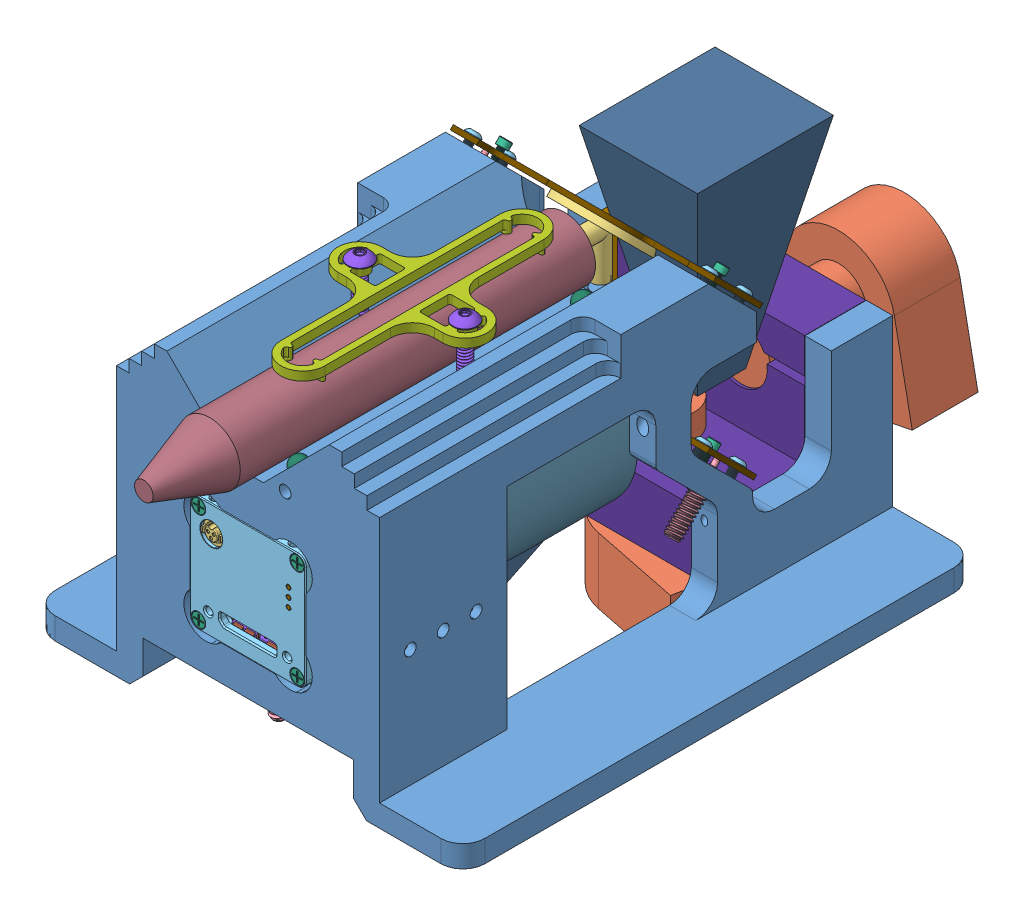
SolidWorks assembly cam_assem, configuration Default. Lengths in mm.
Overall size (98 2576.27 1000).
86 component instances, 46 part files, 77 mates.
Components (placement in the parent):
- cam_holder-1: cam_holder [Default] at origin size (98 71.23 117)
- STP-MQ-(MQ022xG-CM)-ASSM-1: STP-MQ-(MQ022xG-CM)-ASSM [Default] at (0 -13.2 12.4876) x (-1 0 0) z (0 0 -1) size (26.4 26.4 30.19)
  - STP-MQ-(MQ022xG-CM)-ASSM.stp-1: STP-MQ-(MQ022xG-CM)-ASSM.stp [Default] at origin size (26.4 26.4 30.19)
    - SUBASSM-MQ-FRONT.stp-1: SUBASSM-MQ-FRONT.stp [Default] x (0 -1 0) z (0 0 1) size (26.4 26.4 14.6)
      - MECH-MQ-FRONT.stp-1: MECH-MQ-FRONT.stp [Default] at (0 0 7.5) x (1 0 0) z (0 0 -1) size (26.4 26.4 7.5)
      - MECH-MQ-CS-C.stp-1: MECH-MQ-CS-C.stp [Default] at (0 0 0.5) x (1 0 0) z (0 0 -1) size (26.4 26.4 5.5)
      - SROB-M2x14-CUST.stp-1: SROB-M2x14-CUST.stp [Default] at (-11.25 11.25 -7.1) size (3 3 14.55)
      - SROB-M2x14-CUST.stp-2: SROB-M2x14-CUST.stp [Default] at (11.25 -11.25 -7.1) size (3 3 14.55)
      - SROB-M2x14-CUST.stp-3: SROB-M2x14-CUST.stp [Default] at (11.25 11.25 -7.1) size (3 3 14.55)
      - SROB-M2x14-CUST.stp-4: SROB-M2x14-CUST.stp [Default] at (-11.25 -11.25 -7.1) size (3 3 14.55)
    - SUBASSM-MQ-REAR.stp-1: SUBASSM-MQ-REAR.stp [Default] at (0 0 -22.584) x (-1 0 0) z (0 0 1) size (26.4 26.4 10.6)
      - MECH-MQ-REAR.stp-1: MECH-MQ-REAR.stp [Default] at (0 0 6.5) x (-1 0 0) z (0 0 -1) size (26.4 26.4 6.5)
      - SROB-M2x10-CUST .stp-1: SROB-M2x10-CUST .stp [Default] at (-11.25 11.25 10.6) x (1 0 0) z (0 0 -1) size (3 3 10.55)
      - SROB-M2x10-CUST .stp-2: SROB-M2x10-CUST .stp [Default] at (11.25 11.25 10.6) x (1 0 0) z (0 0 -1) size (3 3 10.55)
      - SROB-M2x10-CUST .stp-3: SROB-M2x10-CUST .stp [Default] at (11.25 -11.25 10.6) x (1 0 0) z (0 0 -1) size (3 3 10.55)
      - SROB-M2x10-CUST .stp-4: SROB-M2x10-CUST .stp [Default] at (-11.25 -11.25 10.6) x (1 0 0) z (0 0 -1) size (3 3 10.55)
      - MECH-MQ-THERMAL-PAD.stp-1: MECH-MQ-THERMAL-PAD.stp [Default] at (-10.5 5.45 4.8) x (0.961741 -0.273959 0) z (0 0 -1) size (20.28 8 0.5)
      - MECH-EMI-GSKT-1.3X2.3X11.stp-1: MECH-EMI-GSKT-1.3X2.3X11.stp [Default] at (0 9.9495 3.45) size (11 1.2 3)
      - MECH-EMI-GSKT-1.3X2.3X11.stp-2: MECH-EMI-GSKT-1.3X2.3X11.stp [Default] at (0 7.0505 3.45) size (11 1.2 3)
      - MECH-LIGHTPIPE-1.63X4.14.stp-1: MECH-LIGHTPIPE-1.63X4.14.stp [Default] at (9.3 -3.5 4.1492) x (-1 0 0) z (0 -1 0) size (1.63 4.14 1.63)
      - MECH-LIGHTPIPE-1.63X4.14.stp-2: MECH-LIGHTPIPE-1.63X4.14.stp [Default] at (9.3 -1.5 4.1492) x (-1 0 0) z (0 -1 0) size (1.63 4.14 1.63)
      - MECH-LIGHTPIPE-1.63X4.14.stp-3: MECH-LIGHTPIPE-1.63X4.14.stp [Default] at (9.3 -5.5 4.1492) x (-1 0 0) z (0 -1 0) size (1.63 4.14 1.63)
    - SUBASSM-MQ-MID-022-CM.stp-1: SUBASSM-MQ-MID-022-CM.stp [Default] at (0 0 -4.5) x (-1 0 0) z (0 0 -1) size (26.4 26.4 11.68)
      - MECH-MQ-MID-022-CM-REV2.stp-1: MECH-MQ-MID-022-CM-REV2.stp [Default] at origin size (26.4 26.4 11.59)
      - MECH-O-RING-22X1-VI370.stp-1: MECH-O-RING-22X1-VI370.stp [Default] at (0 0 1.3) x (1 0 0) z (0 1 0) size (24 1 24)
      - FLT-BK7-AR2X-D25.stp-1: FLT-BK7-AR2X-D25.stp [Default] at (0 0 -0.1) size (25 25 1.1)
      - MECH-MX022xG-CM-GSKT.stp-1: MECH-MX022xG-CM-GSKT.stp [Default] at (0 0 3.364) x (0 -1 0) z (0 0 1) size (12.2 17.4 1.27)
    - MQ022xG-CM-PCA-LW_MODEL.stp-1: MQ022xG-CM-PCA-LW_MODEL.stp [Default] at (0 0 -16.486) x (-1 0 0) z (0 0 -1) size (25.43 25.43 13.85)
      - CMV2000.stp-1: CMV2000.stp [Default] at (-0.0259 -0.5261 -1.002) x (-1 0 0) z (0 0 -1) size (18.65 13.5 6.65)
        - ANDON-96UPGA-Socket.stp-1: ANDON-96UPGA-Socket.stp [Default] at origin size (15.9 10.8 3.23)
        - CMV2000_Package.stp-1: CMV2000_Package.stp [Default] at (0 0 3.29) x (-1 0 0) z (0 0 1) size (18.65 13.5 5.45)
        - CMV2000_Glass.stp-1: CMV2000_Glass.stp [Default] at (0 0 6.1) size (18.06 12.95 0.55)
      - MQ022xG-CM-PCA-LW_MODEL-0.stp-1: MQ022xG-CM-PCA-LW_MODEL-0.stp [Default] at origin size (0.25 1.57 4.1)
      - MQ022xG-CM-PCA-LW_MODEL-1.stp-1: MQ022xG-CM-PCA-LW_MODEL-1.stp [Default] at origin size (12.85 2.05 3.8)
      - MQ022xG-CM-PCA-LW_MODEL-2.stp-1: MQ022xG-CM-PCA-LW_MODEL-2.stp [Default] at origin size (25.43 25.43 1)
      - MQ022xG-CM-PCA-LW_MODEL-3.stp-1: MQ022xG-CM-PCA-LW_MODEL-3.stp [Default] at origin size (0.25 1.57 4.1)
      - MQ022xG-CM-PCA-LW_MODEL-4.stp-1: MQ022xG-CM-PCA-LW_MODEL-4.stp [Default] at origin size (5 5 8.1)
      - MQ022xG-CM-PCA-LW_MODEL-5.stp-1: MQ022xG-CM-PCA-LW_MODEL-5.stp [Default] at origin size (0.25 1.57 4.1)
      - MQ022xG-CM-PCA-LW_MODEL-6.stp-1: MQ022xG-CM-PCA-LW_MODEL-6.stp [Default] at origin size (0.25 1.57 4.1)
      - MQ022xG-CM-PCA-LW_MODEL-7.stp-1: MQ022xG-CM-PCA-LW_MODEL-7.stp [Default] at origin size (0.25 1.57 4.1)
      - MQ022xG-CM-PCA-LW_MODEL-8.stp-1: MQ022xG-CM-PCA-LW_MODEL-8.stp [Default] at origin size (0.25 1.57 4.1)
      - MQ022xG-CM-PCA-LW_MODEL-9.stp-1: MQ022xG-CM-PCA-LW_MODEL-9.stp [Default] at origin size (0.25 1.57 4.1)
      - MQ022xG-CM-PCA-LW_MODEL-10.stp-1: MQ022xG-CM-PCA-LW_MODEL-10.stp [Default] at origin size (0.25 1.57 4.1)
      - MQ022xG-CM-PCA-LW_MODEL-11.stp-1: MQ022xG-CM-PCA-LW_MODEL-11.stp [Default] at origin size (0.25 1.57 4.1)
      - MQ022xG-CM-PCA-LW_MODEL-12.stp-1: MQ022xG-CM-PCA-LW_MODEL-12.stp [Default] at origin size (13.8 3 5.6)
      - MQ022xG-CM-PCA-LW_MODEL-13.stp-1: MQ022xG-CM-PCA-LW_MODEL-13.stp [Default] at origin size (0.25 1.57 4.1)
- laser-1: laser [Default] at (0 18.5208 -37.2385) x (0 -1 0) z (0 0 1) size (14 14 96)
- lens-1: lens [Default] at (0 -13.2 -37.0124) x (0 1 0) z (0 0 1) size (33.5 33.5 46.47)
- 1598K25_Hardened Bearing-Quality 440C Stainless Steel Ball-1: 1598K25_Hardened Bearing-Quality 440C Stainless Steel Ball [1598K25] at (-6.6608 12.5671 30) x (0.595435 0.636273 0.490525) z (-0.571952 -0.093063 0.814991) size (4 4 4)
- 92695A729_Alloy Steel Cone-Point Set Screws-1: 92695A729_Alloy Steel Cone-Point Set Screws [92695A729] at (-8.4853 10.8376 24.4029) x (0.913011 -0.407935 0) z (0 0 1) size (4.05 3.54 3.43)
- 1598K25_Hardened Bearing-Quality 440C Stainless Steel Ball-2: 1598K25_Hardened Bearing-Quality 440C Stainless Steel Ball [1598K25] at (-6.364 12.1569 -35) x (0.756378 0.1991 0.623098) z (-0.446406 -0.539153 0.714168) size (4 4 4)
- 1598K25_Hardened Bearing-Quality 440C Stainless Steel Ball-4: 1598K25_Hardened Bearing-Quality 440C Stainless Steel Ball [1598K25] at (6.364 12.1569 -35) x (0.295652 0.723786 0.623477) z (-0.259043 -0.567459 0.781593) size (4 4 4)
- galvo_block-1: galvo_block [Default] at (-18.725 -27.865 -82) x (0 -1 0) z (1 0 0) size (39.65 34.73 42.65)
- D_holder-1: D_holder [Default] at (0 -12.8464 -45.6926) x (1 0 0) z (0 -0.707107 0.707107) size (60 27.4 1)
- D-1: D [Default] at (0 -13.2 -45.339) x (1 0 0) z (0 -0.707107 0.707107) size (20 121.63 78.36)
- glavo-1: glavo [Default] at (0 -59.1765 -60.255) x (0.199368 0 -0.979925) z (0.979925 0 0.199368) size (26 51 34)
- D_holder-2: D_holder [Default] at (0 20.2886 -47.1068) x (1 0 0) z (0 -0.707107 0.707107) size (60 27.4 1)
- mirror-1: mirror [Default] at (0 18.5208 -45.339) x (-1 0 0) z (0 0.707107 -0.707107) size (20 121.63 78.36)
- 3126A21_Slotted Long-Nose Steel Spring Plunger-1: 3126A21_Slotted Long-Nose Steel Spring Plunger [3126A21] at (27 -19.2382 -39.3008) x (0.917455 -0.281315 -0.281315) z (0.397839 0.648739 0.648739) size (3.52 15.42 3.68)
- 92949A319_18-8 Stainless Steel Button Head Hex Drive Screw-1: 92949A319_18-8 Stainless Steel Button Head Hex Drive Screw [92949A319] at (27 -10.9061 -39.8548) x (-0.780279 -0.442247 -0.442247) z (0 0.707107 -0.707107) size (3.28 3.28 7.4)
- 92196A051_18-8 Stainless Steel Socket Head Screw-1: 92196A051_18-8 Stainless Steel Socket Head Screw [92196A051] at (24.75 -13.1743 -45.3647) x (-0.756852 -0.462156 -0.462156) z (0 0.707107 -0.707107) size (2.44 2.44 4.07)
- 92949A319_18-8 Stainless Steel Button Head Hex Drive Screw-2: 92949A319_18-8 Stainless Steel Button Head Hex Drive Screw [92949A319] at (27 -18.6842 -47.633) x (-0.793626 -0.430208 -0.430208) z (0 0.707107 -0.707107) size (3.28 3.28 7.4)
- 92949A319_18-8 Stainless Steel Button Head Hex Drive Screw-3: 92949A319_18-8 Stainless Steel Button Head Hex Drive Screw [92949A319] at (-27 -10.9061 -39.8548) x (-0.831896 -0.392395 -0.392395) z (0 0.707107 -0.707107) size (3.28 3.28 7.4)
- 92949A319_18-8 Stainless Steel Button Head Hex Drive Screw-4: 92949A319_18-8 Stainless Steel Button Head Hex Drive Screw [92949A319] at (-27 -18.6842 -47.633) x (-0.88833 -0.324707 -0.324707) z (0 0.707107 -0.707107) size (3.28 3.28 7.4)
- 92196A051_18-8 Stainless Steel Socket Head Screw-2: 92196A051_18-8 Stainless Steel Socket Head Screw [92196A051] at (-24.75 -13.1164 -45.4227) x (-0.770813 -0.45047 -0.45047) z (0 0.707107 -0.707107) size (2.44 2.44 4.07)
- 3126A21_Slotted Long-Nose Steel Spring Plunger-3: 3126A21_Slotted Long-Nose Steel Spring Plunger [3126A21] at (-27 -19.4685 -39.0705) x (0.908634 -0.295283 -0.295283) z (0.417593 0.642502 0.642502) size (3.52 15.42 3.68)
- 3126A21_Slotted Long-Nose Steel Spring Plunger-5: 3126A21_Slotted Long-Nose Steel Spring Plunger [3126A21] at (-27 13.9393 -40.5359) x (0.687618 -0.513411 -0.513411) z (0.726072 0.48622 0.48622) size (3.52 15.42 3.68)
- 92949A319_18-8 Stainless Steel Button Head Hex Drive Screw-7: 92949A319_18-8 Stainless Steel Button Head Hex Drive Screw [92949A319] at (27 22.229 -41.269) x (-0.793626 -0.430208 -0.430208) z (0 0.707107 -0.707107) size (3.28 3.28 7.4)
- 92949A319_18-8 Stainless Steel Button Head Hex Drive Screw-10: 92949A319_18-8 Stainless Steel Button Head Hex Drive Screw [92949A319] at (27 14.4508 -49.0472) x (-0.806602 -0.417967 -0.417967) z (0 0.707107 -0.707107) size (3.28 3.28 7.4)
- 92949A319_18-8 Stainless Steel Button Head Hex Drive Screw-11: 92949A319_18-8 Stainless Steel Button Head Hex Drive Screw [92949A319] at (-27 22.229 -41.269) x (-0.843706 -0.379579 -0.379579) z (0 0.707107 -0.707107) size (3.28 3.28 7.4)
- 92949A319_18-8 Stainless Steel Button Head Hex Drive Screw-12: 92949A319_18-8 Stainless Steel Button Head Hex Drive Screw [92949A319] at (-27 14.4508 -49.0472) x (-0.898056 -0.311043 -0.311043) z (0 0.707107 -0.707107) size (3.28 3.28 7.4)
- 92196A051_18-8 Stainless Steel Socket Head Screw-4: 92196A051_18-8 Stainless Steel Socket Head Screw [92196A051] at (24.75 20.4716 -47.2898) x (-0.770813 -0.45047 -0.45047) z (0 0.707107 -0.707107) size (2.44 2.44 4.07)
- 92196A051_18-8 Stainless Steel Socket Head Screw-6: 92196A051_18-8 Stainless Steel Socket Head Screw [92196A051] at (-24.75 20.4716 -47.2898) x (-0.784414 -0.438574 -0.438574) z (0 0.707107 -0.707107) size (2.44 2.44 4.07)
- 3126A21_Slotted Long-Nose Steel Spring Plunger-7: 3126A21_Slotted Long-Nose Steel Spring Plunger [3126A21] at (0 -34.7439 28) size (3.52 15.42 3.68)
- 3126A21_Slotted Long-Nose Steel Spring Plunger-8: 3126A21_Slotted Long-Nose Steel Spring Plunger [3126A21] at (0 -34.7439 13) x (0.982082 0 -0.188455) z (0.188455 0 0.982082) size (3.52 15.42 3.68)
- 3126A21_Slotted Long-Nose Steel Spring Plunger-10: 3126A21_Slotted Long-Nose Steel Spring Plunger [3126A21] at (21.5439 -13.2 28) x (0 0.999599 -0.02833) z (0 0.02833 0.999599) size (3.52 15.42 3.68)
- 3126A21_Slotted Long-Nose Steel Spring Plunger-12: 3126A21_Slotted Long-Nose Steel Spring Plunger [3126A21] at (21.5439 -13.2 13) x (0 0.991446 0.130517) z (0 -0.130517 0.991446) size (3.52 15.42 3.68)
- clamp-1: clamp [Default] at (0 27.583 -2.5) x (0 0 -1) z (-1 0 0) size (60 3 34)
- 92949A113_18-8 Stainless Steel Button Head Hex Drive Screw-1: 92949A113_18-8 Stainless Steel Button Head Hex Drive Screw [92949A113] at (12 18.8073 -2.5) x (-0.837169 0 -0.546944) z (0 1 0) size (5.41 5.41 20.93)
- 92949A113_18-8 Stainless Steel Button Head Hex Drive Screw-2: 92949A113_18-8 Stainless Steel Button Head Hex Drive Screw [92949A113] at (-12 18.8073 -2.5) x (-0.925243 0 -0.379375) z (0 1 0) size (5.41 5.41 20.93)
- 1598K25_Hardened Bearing-Quality 440C Stainless Steel Ball-6: 1598K25_Hardened Bearing-Quality 440C Stainless Steel Ball [1598K25] at (6.7083 12.5196 30) x (-0.036454 0.98158 0.187543) z (-0.758508 -0.149364 0.634315) size (4 4 4)
- 92695A729_Alloy Steel Cone-Point Set Screws-2: 92695A729_Alloy Steel Cone-Point Set Screws [92695A729] at (8.4729 10.7426 24.2676) x (0.992207 -0.1246 0) z (0 0 1) size (4.05 3.54 3.43)
- glavo-2: glavo [Default] at (9 -13.2 -105.6229) x (0.980901 0.194509 0) z (0.194509 -0.980901 0) size (26 51 34)
- spacer-1: spacer [Default] at (-24.005 -27.865 -82) x (0 -1 0) z (1 0 0) size (39.65 34.73 5.28)
- beam-1: beam [Default] at (9.2842 -13.1356 -60.207) size (26.98 50 30.98)
- beam-2: beam [Default] at (-0.2804 -13.3696 -59.6494) x (1 0 0) z (0 -0.999962 0.008727) size (26.98 50 30.98)
Mates (geometry in assembly coordinates):
- Coincident2: coincident anti-aligned: plane of STP-MQ-(MQ022xG-CM)-ASSM-1 through (0 -13.2 12.4876) normal (-1 0 0)
- Concentric2: concentric: cylinder of cam_holder-1 through (-8.4853 10.7426 30) axis (0.707107 0.707107 0) radius 2; sphere of 1598K25_Hardened Bearing-Quality 440C Stainless Steel Ball-1
- Concentric5: concentric aligned: cylinder of STP-MQ-(MQ022xG-CM)-ASSM-1/STP-MQ-(MQ022xG-CM)-ASSM.stp-1/SUBASSM-MQ-FRONT.stp-1/MECH-MQ-FRONT.stp-1 through (0 -13.2 11.4876) axis (0 0 -1) radius 12.2703; cylinder of lens-1 through (0 -13.2 9.4576) axis (0 0 -1) radius 12.65
- Coincident3: coincident anti-aligned: plane of STP-MQ-(MQ022xG-CM)-ASSM-1/STP-MQ-(MQ022xG-CM)-ASSM.stp-1/SUBASSM-MQ-FRONT.stp-1/MECH-MQ-FRONT.stp-1 through (-13.2 0 4.9876) normal (0 0 -1); plane of lens-1 through (0 -13.2 4.9876) normal (0 0 1)
- Coincident4: coincident anti-aligned: plane of cam_holder-1 through (-13.2 0 35) normal (0 -1 0); plane of STP-MQ-(MQ022xG-CM)-ASSM-1/STP-MQ-(MQ022xG-CM)-ASSM.stp-1/SUBASSM-MQ-MID-022-CM.stp-1/MECH-MQ-MID-022-CM-REV2.stp-1 through (13.2 0 28.5716) normal (0 1 0)
- Parallel1: parallel aligned: plane of lens-1 through (0 -13.2 -37.0124) normal (0 1 0)
- Coincident7: coincident aligned: plane of lens-1 through (0 -13.2 -37.0124) normal (0 1 0); plane of galvo_block-1 through (-18.725 -13.2 -82) normal (0 1 0)
- Coincident8: coincident: plane of cam_holder-1 through (0 0 0) normal (0 0 -1); plane of lens-1 through (0 -13.2 0) normal (0 0 1)
- Coincident9: coincident aligned: plane of lens-1 through (0 -13.2 -37.0124) normal (-1 0 0); plane of galvo_block-1 through (0 -27.865 -82) normal (-1 0 0)
- Coincident10: coincident aligned: plane of cam_holder-1 through (0 0 -82) normal (0 0 -1); plane of galvo_block-1 through (23.925 -27.865 -82) normal (0 0 -1)
- Concentric6: concentric anti-aligned: cylinder of D_holder-1 through (0 -13.2 -45.339) axis (0 -0.707107 0.707107) radius 10.1; cylinder of D-1 through (0 -14.6142 -43.9248) axis (0 0.707107 -0.707107) radius 10
- Coincident12: coincident anti-aligned: plane of D_holder-1 through (0 -13.2 -45.339) normal (0 -0.707107 0.707107); plane of D-1 through (0 -13.2 -45.339) normal (0 0.707107 -0.707107)
- Coincident14: coincident aligned: plane of lens-1 through (0 -13.2 -37.0124) normal (0 1 0); plane of D_holder-1 through (0 -13.2 -45.6926) normal (0 1 0)
- Coincident15: coincident anti-aligned: plane of lens-1 through (0 -13.2 -37.0124) normal (-1 0 0); plane of D_holder-1 through (0 -12.8464 -45.6926) normal (1 0 0)
- Concentric7: concentric anti-aligned: cylinder of galvo_block-1 through (0 -70.515 -60.255) axis (0 1 0) radius 6.425; cylinder of glavo-1 through (0 -22.1765 -60.255) axis (0 -1 0) radius 6.5
- Concentric8: concentric aligned: cylinder of D_holder-2 through (0 19.935 -46.7533) axis (0 -0.707107 0.707107) radius 10.1; cylinder of mirror-1 through (0 19.935 -46.7533) axis (0 -0.707107 0.707107) radius 10
- Coincident16: coincident anti-aligned: plane of D_holder-2 through (0 19.935 -46.7533) normal (0 -0.707107 0.707107); plane of mirror-1 through (0 19.935 -46.7533) normal (0 0.707107 -0.707107)
- Concentric9: concentric aligned: cylinder of laser-1 through (0 18.5208 58.7615) axis (0 0 -1) radius 7; axis of mirror-1 through (0 18.5208 -25.339) axis (0 0 -1)
- Coincident17: coincident aligned: plane of laser-1 through (0 18.5208 -37.2385) normal (1 0 0)
- Parallel2: parallel anti-aligned: plane of laser-1 through (0 18.5208 -37.2385) normal (0 -1 0)
- Parallel3: parallel anti-aligned: plane of cam_holder-1 through (49 8 -57) normal (0 0.707107 -0.707107); plane of D_holder-2 through (0 19.5815 -46.3997) normal (0 -0.707107 0.707107)
- Coincident20: coincident aligned: plane of D_holder-2 through (0 20.2886 -47.1068) normal (1 0 0)
- Concentric10: concentric anti-aligned: cylinder of D-1 through (0 6.8 -45.339) axis (0 -1 0) radius 2; cylinder of mirror-1 through (0 8.5208 -45.339) axis (0 1 0) radius 2
- Concentric11: concentric aligned: cylinder of cam_holder-1 through (27 -14.5551 -43.984) axis (0 0.707107 -0.707107) radius 1.3526; cylinder of 3126A21_Slotted Long-Nose Steel Spring Plunger-1 through (27 -13.3382 -45.2008) axis (0 0.707107 -0.707107) radius 0.5715
- Concentric12: concentric aligned: cylinder of D_holder-1 through (27 -8.9574 -41.8035) axis (0 0.707107 -0.707107) radius 1.1303; cylinder of 92949A319_18-8 Stainless Steel Button Head Hex Drive Screw-1 through (27 -8.3647 -42.3962) axis (0 0.707107 -0.707107) radius 1.6383
- Coincident21: coincident anti-aligned: plane of D_holder-1 through (0 -12.8464 -45.6926) normal (0 0.707107 -0.707107); plane of 92949A319_18-8 Stainless Steel Button Head Hex Drive Screw-1 through (25.9754 -8.0534 -40.8996) normal (0 -0.707107 0.707107)
- Concentric13: concentric anti-aligned: cylinder of D_holder-1 through (24.75 -12.8464 -45.6926) axis (0 0.707107 -0.707107) radius 0.5956; cylinder of 92196A051_18-8 Stainless Steel Socket Head Screw-1 through (24.75 -14.5551 -43.984) axis (0 -0.707107 0.707107) radius 1.2192
- Concentric14: concentric aligned: cylinder of cam_holder-1 through (27 -10.666 -40.0949) axis (0 0.707107 -0.707107) radius 0.7556; cylinder of 92949A319_18-8 Stainless Steel Button Head Hex Drive Screw-1 through (27 -8.3647 -42.3962) axis (0 0.707107 -0.707107) radius 1.6383
- Coincident22: coincident anti-aligned: plane of cam_holder-1 through (49 -20.0563 -49.4853) normal (0 0.707107 -0.707107); plane of 92196A051_18-8 Stainless Steel Socket Head Screw-1 through (24.4076 -14.2747 -43.7036) normal (0 -0.707107 0.707107)
- Concentric15: concentric aligned: cylinder of D_holder-1 through (27 -16.7355 -49.5817) axis (0 0.707107 -0.707107) radius 1.1303; cylinder of 92949A319_18-8 Stainless Steel Button Head Hex Drive Screw-2 through (27 -16.1428 -50.1744) axis (0 0.707107 -0.707107) radius 1.6383
- Coincident23: coincident anti-aligned: plane of D_holder-1 through (0 -12.8464 -45.6926) normal (0 0.707107 -0.707107); plane of 92949A319_18-8 Stainless Steel Button Head Hex Drive Screw-2 through (26.0032 -15.8162 -48.6623) normal (0 -0.707107 0.707107)
- Concentric16: concentric aligned: cylinder of D_holder-1 through (-27 -8.9574 -41.8035) axis (0 0.707107 -0.707107) radius 1.1303; cylinder of 92949A319_18-8 Stainless Steel Button Head Hex Drive Screw-3 through (-27 -8.3647 -42.3962) axis (0 0.707107 -0.707107) radius 1.6383
- Coincident26: coincident anti-aligned: plane of D_holder-1 through (0 -12.8464 -45.6926) normal (0 0.707107 -0.707107); plane of 92949A319_18-8 Stainless Steel Button Head Hex Drive Screw-3 through (-27.9091 -7.9936 -40.8398) normal (0 -0.707107 0.707107)
- Coincident27: coincident anti-aligned: plane of D_holder-1 through (0 -12.8464 -45.6926) normal (0 0.707107 -0.707107); plane of 92949A319_18-8 Stainless Steel Button Head Hex Drive Screw-4 through (-27.7523 -15.7064 -48.5526) normal (0 -0.707107 0.707107)
- Concentric17: concentric aligned: cylinder of D_holder-1 through (-27 -16.7355 -49.5817) axis (0 0.707107 -0.707107) radius 1.1303; cylinder of 92949A319_18-8 Stainless Steel Button Head Hex Drive Screw-4 through (-27 -16.1428 -50.1744) axis (0 0.707107 -0.707107) radius 1.6383
- Concentric18: concentric anti-aligned: cylinder of D_holder-1 through (-24.75 -12.8464 -45.6926) axis (0 0.707107 -0.707107) radius 0.5956; cylinder of 92196A051_18-8 Stainless Steel Socket Head Screw-2 through (-24.75 -14.4971 -44.0419) axis (0 -0.707107 0.707107) radius 1.2192
- Concentric19: concentric aligned: cylinder of cam_holder-1 through (-27 -14.5551 -43.984) axis (0 0.707107 -0.707107) radius 1.3526; cylinder of 3126A21_Slotted Long-Nose Steel Spring Plunger-3 through (-27 -13.5685 -44.9705) axis (0 0.707107 -0.707107) radius 0.5715
- Concentric20: concentric aligned: cylinder of cam_holder-1 through (-27 19.2017 -45.7983) axis (0 0.707107 -0.707107) radius 1.3526; cylinder of 3126A21_Slotted Long-Nose Steel Spring Plunger-5 through (-27 19.8394 -46.4359) axis (0 0.707107 -0.707107) radius 0.5715
- Concentric22: concentric aligned: cylinder of D_holder-2 through (27 24.1777 -43.2177) axis (0 0.707107 -0.707107) radius 1.1303; cylinder of 92949A319_18-8 Stainless Steel Button Head Hex Drive Screw-7 through (27 24.7704 -43.8104) axis (0 0.707107 -0.707107) radius 1.6383
- Coincident29: coincident anti-aligned: plane of D_holder-2 through (0 20.2886 -47.1068) normal (0 0.707107 -0.707107); plane of 92949A319_18-8 Stainless Steel Button Head Hex Drive Screw-7 through (26.0032 25.097 -42.2983) normal (0 -0.707107 0.707107)
- Concentric24: concentric aligned: cylinder of D_holder-2 through (27 16.3995 -50.9959) axis (0 0.707107 -0.707107) radius 1.1303; cylinder of 92949A319_18-8 Stainless Steel Button Head Hex Drive Screw-10 through (27 16.9922 -51.5886) axis (0 0.707107 -0.707107) radius 1.6383
- Coincident31: coincident anti-aligned: plane of D_holder-2 through (0 20.2886 -47.1068) normal (0 0.707107 -0.707107); plane of 92949A319_18-8 Stainless Steel Button Head Hex Drive Screw-10 through (26.0316 17.3339 -50.0615) normal (0 -0.707107 0.707107)
- Coincident32: coincident anti-aligned: plane of D_holder-2 through (0 20.2886 -47.1068) normal (0 0.707107 -0.707107); plane of 92949A319_18-8 Stainless Steel Button Head Hex Drive Screw-11 through (-27.8794 25.1551 -42.2403) normal (0 -0.707107 0.707107)
- Concentric25: concentric aligned: cylinder of D_holder-2 through (-27 24.1777 -43.2177) axis (0 0.707107 -0.707107) radius 1.1303; cylinder of 92949A319_18-8 Stainless Steel Button Head Hex Drive Screw-11 through (-27 24.7704 -43.8104) axis (0 0.707107 -0.707107) radius 1.6383
- Coincident33: coincident anti-aligned: plane of D_holder-2 through (0 20.2886 -47.1068) normal (0 0.707107 -0.707107); plane of 92949A319_18-8 Stainless Steel Button Head Hex Drive Screw-12 through (-27.7207 17.4399 -49.9555) normal (0 -0.707107 0.707107)
- Concentric26: concentric aligned: cylinder of D_holder-2 through (-27 16.3995 -50.9959) axis (0 0.707107 -0.707107) radius 1.1303; cylinder of 92949A319_18-8 Stainless Steel Button Head Hex Drive Screw-12 through (-27 16.9922 -51.5886) axis (0 0.707107 -0.707107) radius 1.6383
- Concentric27: concentric anti-aligned: cylinder of D_holder-2 through (24.75 20.2886 -47.1068) axis (0 0.707107 -0.707107) radius 0.5956; cylinder of 92196A051_18-8 Stainless Steel Socket Head Screw-4 through (24.75 19.0909 -45.9091) axis (0 -0.707107 0.707107) radius 1.2192
- Coincident36: coincident anti-aligned: plane of cam_holder-1 through (49 8 -57) normal (0 0.707107 -0.707107); plane of 92196A051_18-8 Stainless Steel Socket Head Screw-4 through (24.4163 19.3764 -45.6236) normal (0 -0.707107 0.707107)
- Concentric28: concentric anti-aligned: cylinder of D_holder-2 through (-24.75 20.2886 -47.1068) axis (0 0.707107 -0.707107) radius 0.5956; cylinder of 92196A051_18-8 Stainless Steel Socket Head Screw-6 through (-24.75 19.0909 -45.9091) axis (0 -0.707107 0.707107) radius 1.2192
- Coincident37: coincident anti-aligned: plane of cam_holder-1 through (49 8 -57) normal (0 0.707107 -0.707107); plane of 92196A051_18-8 Stainless Steel Socket Head Screw-6 through (-25.0749 19.3815 -45.6185) normal (0 -0.707107 0.707107)
- Concentric29: concentric anti-aligned: cylinder of cam_holder-1 through (0 -34.4 28) axis (0 -1 0) radius 1.3526; line of 3126A21_Slotted Long-Nose Steel Spring Plunger-7 through (0 -27.3144 28) axis (0 1 0)
- Tangent6: tangent anti-aligned: plane of STP-MQ-(MQ022xG-CM)-ASSM-1/STP-MQ-(MQ022xG-CM)-ASSM.stp-1/SUBASSM-MQ-MID-022-CM.stp-1/MECH-MQ-MID-022-CM-REV2.stp-1 through (-13.2 -26.4 28.5716) normal (0 -1 0); sphere of 3126A21_Slotted Long-Nose Steel Spring Plunger-7
- Concentric30: concentric anti-aligned: cylinder of cam_holder-1 through (0 -34.4 13) axis (0 -1 0) radius 1.3526; line of 3126A21_Slotted Long-Nose Steel Spring Plunger-8 through (0 -27.3144 13) axis (0 1 0)
- Tangent7: tangent anti-aligned: plane of STP-MQ-(MQ022xG-CM)-ASSM-1/STP-MQ-(MQ022xG-CM)-ASSM.stp-1/SUBASSM-MQ-MID-022-CM.stp-1/MECH-MQ-MID-022-CM-REV2.stp-1 through (-13.2 -26.4 28.5716) normal (0 -1 0); sphere of 3126A21_Slotted Long-Nose Steel Spring Plunger-8
- Concentric31: concentric anti-aligned: cylinder of cam_holder-1 through (30 -13.2 28) axis (1 0 0) radius 1.3526; line of 3126A21_Slotted Long-Nose Steel Spring Plunger-10 through (14.1144 -13.2 28) axis (-1 0 0)
- Tangent9: tangent anti-aligned: plane of STP-MQ-(MQ022xG-CM)-ASSM-1/STP-MQ-(MQ022xG-CM)-ASSM.stp-1/SUBASSM-MQ-REAR.stp-1/MECH-MQ-REAR.stp-1 through (13.2 -26.4 35.0716) normal (1 0 0); sphere of 3126A21_Slotted Long-Nose Steel Spring Plunger-10
- Concentric32: concentric anti-aligned: cylinder of cam_holder-1 through (30 -13.2 13) axis (1 0 0) radius 1.3526; line of 3126A21_Slotted Long-Nose Steel Spring Plunger-12 through (14.1144 -13.2 13) axis (-1 0 0)
- Tangent10: tangent anti-aligned: plane of STP-MQ-(MQ022xG-CM)-ASSM-1/STP-MQ-(MQ022xG-CM)-ASSM.stp-1/SUBASSM-MQ-REAR.stp-1/MECH-MQ-REAR.stp-1 through (13.2 -26.4 35.0716) normal (1 0 0); sphere of 3126A21_Slotted Long-Nose Steel Spring Plunger-12
- Concentric33: concentric: cylinder of assembly; line of assembly; cylinder of cam_holder-1 through (-12 15 -2.5) axis (0 1 0) radius 1.1303; axis of clamp-1 through (-12 25.583 -2.5) axis (0 1 0)
- Parallel4: parallel aligned: plane of cam_holder-1 through (-30 -40 35) normal (-1 0 0); plane of clamp-1 through (-5 25.583 22.5) normal (-1 0 0)
- Tangent14: tangent: cylinder of laser-1 through (0 18.5208 58.7615) axis (0 0 -1) radius 7; circle of clamp-1
- Concentric36: concentric aligned: cylinder of clamp-1 through (12 27.583 -2.5) axis (0 1 0) radius 1.4732; cylinder of 92949A113_18-8 Stainless Steel Button Head Hex Drive Screw-1 through (12 29.0816 -2.5) axis (0 1 0) radius 2.7051
- Coincident40: coincident anti-aligned: plane of clamp-1 through (0 27.583 22.5) normal (0 1 0); plane of 92949A113_18-8 Stainless Steel Button Head Hex Drive Screw-1 through (10.5205 27.583 -0.2354) normal (0 -1 0)
- Concentric37: concentric aligned: cylinder of clamp-1 through (-12 27.583 -2.5) axis (0 1 0) radius 1.4732; cylinder of 92949A113_18-8 Stainless Steel Button Head Hex Drive Screw-2 through (-12 29.0816 -2.5) axis (0 1 0) radius 2.7051
- Coincident41: coincident anti-aligned: plane of clamp-1 through (0 27.583 22.5) normal (0 1 0); plane of 92949A113_18-8 Stainless Steel Button Head Hex Drive Screw-2 through (-13.0262 27.583 0.0029) normal (0 -1 0)
- Concentric38: concentric: cylinder of cam_holder-1 through (-7.7782 10.7426 -35) axis (0.707107 0.707107 0) radius 2; sphere of 1598K25_Hardened Bearing-Quality 440C Stainless Steel Ball-2
- Tangent16: tangent: plane of cam_holder-1 through (-7.7782 10.7426 -35) normal (0.707107 0.707107 0); sphere of 1598K25_Hardened Bearing-Quality 440C Stainless Steel Ball-2
- Concentric39: concentric: cylinder of cam_holder-1 through (7.7782 10.7426 -35) axis (-0.707107 0.707107 0) radius 2; sphere of 1598K25_Hardened Bearing-Quality 440C Stainless Steel Ball-4
- Tangent18: tangent: plane of cam_holder-1 through (7.7782 10.7426 -35) normal (-0.707107 0.707107 0); sphere of 1598K25_Hardened Bearing-Quality 440C Stainless Steel Ball-4
- Concentric41: concentric: cylinder of cam_holder-1 through (8.4853 10.7426 30) axis (-0.707107 0.707107 0) radius 2; sphere of 1598K25_Hardened Bearing-Quality 440C Stainless Steel Ball-6
- Tangent19: tangent aligned: cylinder of cam_holder-1 through (8.4853 10.7426 35) axis (0 0 1) radius 1.3526; face of 92695A729_Alloy Steel Cone-Point Set Screws-2
- Tangent20: tangent anti-aligned: cylinder of laser-1 through (0 18.5208 58.7615) axis (0 0 -1) radius 7; sphere of 1598K25_Hardened Bearing-Quality 440C Stainless Steel Ball-4
- Concentric42: concentric anti-aligned: cylinder of galvo_block-1 through (9 -13.2 -110.65) axis (0 0 1) radius 6.425; cylinder of glavo-2 through (9 -13.2 -68.6229) axis (0 0 -1) radius 6.5
- Coincident42: coincident aligned: plane of galvo_block-1 through (23.925 -27.865 -82) normal (0 0 -1); plane of spacer-1 through (18.645 -27.865 -82) normal (0 0 -1)
- Coincident43: coincident anti-aligned: plane of galvo_block-1 through (-18.725 -27.865 -82) normal (-1 0 0); plane of spacer-1 through (-18.725 8.5536 -47.27) normal (1 0 0)
- Coincident44: coincident aligned: plane of galvo_block-1 through (23.925 -41.865 -82) normal (0 -1 0); plane of spacer-1 through (18.645 -41.865 -82) normal (0 -1 0)
- Angle1: planar angle = 0.200713 rad aligned: plane of galvo_block-1 through (23.925 -27.865 -82) normal (0 0 -1); plane of glavo-1 through (23.1702 -44.1765 -68.8073) normal (0.199368 0 -0.979925)
